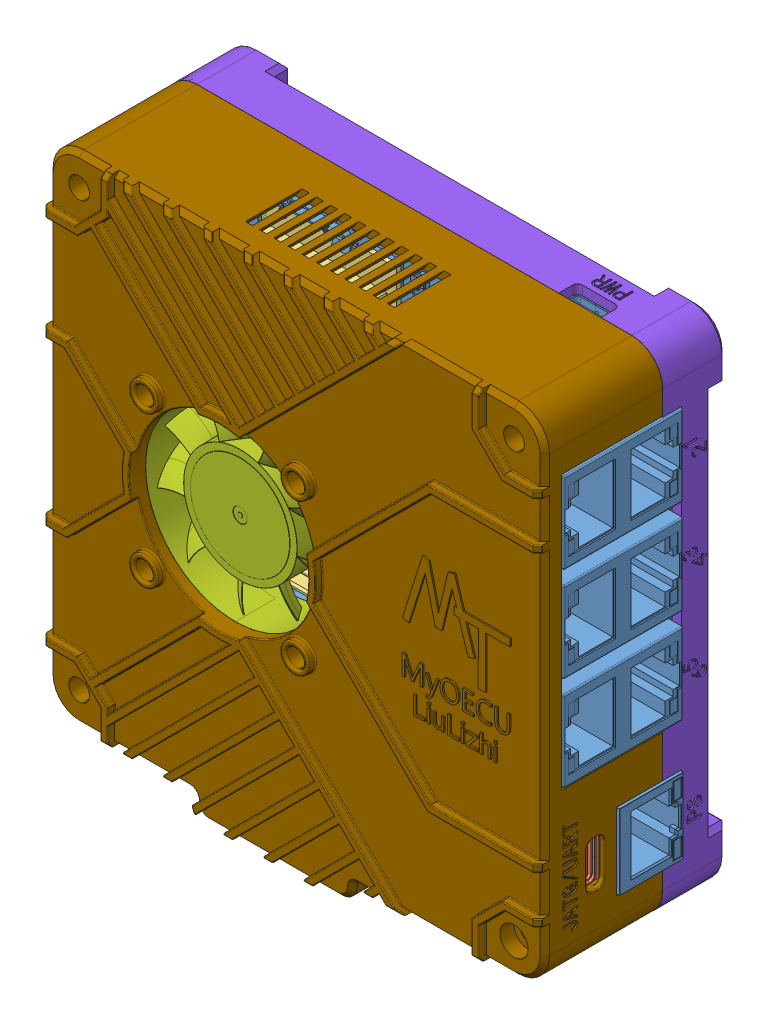
SolidWorks assembly MyOECU_装配1, configuration 默认. Lengths in mm.
Overall size (110.76 109.2 40.07).
11 component instances, 9 part files, 21 mates.
Components (placement in the parent):
- OECU_BASE-1: OECU_BASE [默认] at (25.1566 -137.4235 46.5251) size (110.76 104.44 29.35)
- JTAG-1: JTAG [默认] at (121.0536 -114.4556 17.2477) size (47.13 32.25 13.3)
- ZYNQ_CORE-1: ZYNQ_CORE [1.5V] at (53.9162 -68.6655 52.5951) x (0 -1 0) z (-1 0 0) size (67.6 9 30)
- Column_M3x16-1: Column_M3x16 [Predeterminado] at (93.1566 -123.4235 52.5251) x (1 0 0) z (0 -1 0) size (5.77 15 5)
- Column_M3x16-2: Column_M3x16 [Predeterminado] at (131.1566 -123.4235 52.5251) x (1 0 0) z (0 -1 0) size (5.77 15 5)
- Column_M3x16-3: Column_M3x16 [Predeterminado] at (131.1566 -99.4235 52.5251) x (1 0 0) z (0 -1 0) size (5.77 15 5)
- PinSocket7_2.54-1: PinSocket7_2.54 [默认] at (87.8883 -116.9162 44.9359) x (0 1 0) z (0 0 -1) size (10.13 17.78 5.84)
- OLED-1: OLED [Default] at (93.9183 -129.4462 69.9659) x (-1 0 0) z (0 0 1) size (27.3 11.8 27.8)
- 4010_FAN-1: 4010_FAN [默认] at (70.1566 -77.4235 62.4359) x (0 -1 0) z (-1 0 0) size (43.27 11 40)
- 外壳_底壳-2: 外壳_底壳 [默认] at (0.001 -127.4235 39.9359) x (1 0 0) z (0 -1 0) size (105 14.95 109.2)
- 外壳_上壳-1: 外壳_上壳 [默认] at (-5.4222 -123.4235 73.4359) x (1 0 0) z (0 -1 0) size (105 30.2 109.2)
Mates (geometry in assembly coordinates):
- 同心2: concentric aligned: cylinder of OECU_BASE-1 through (131.1566 -123.4235 44.9359) axis (0 0 -1) radius 1.6; cylinder of JTAG-1 through (131.1566 -123.4235 61.5251) axis (0 0 -1) radius 1.6
- 重合2: coincident: plane of OECU_BASE-1 through (55.9626 -100.8705 52.0951) normal (0 0 1); plane of ZYNQ_CORE-1 through (83.9162 -34.8655 52.0951) normal (0 0 -1)
- 重合3: coincident anti-aligned: plane of OECU_BASE-1 through (49.1126 -60.1655 54.5751) normal (0 -1 0); plane of ZYNQ_CORE-1 through (53.9162 -60.1655 52.0951) normal (0 1 0)
- 重合4: coincident anti-aligned: plane of OECU_BASE-1 through (39.1566 -127.4235 46.5251) normal (0 0 1); plane of Column_M3x16-1 through (93.1566 -123.4235 46.5251) normal (0 0 -1)
- 同心3: concentric aligned: cylinder of JTAG-1 through (93.1566 -123.4235 61.5251) axis (0 0 -1) radius 1.6; cylinder of Column_M3x16-1 through (93.1566 -123.4235 58.5251) axis (0 0 -1) radius 1.5
- 同心4: concentric aligned: cylinder of JTAG-1 through (131.1566 -123.4235 61.5251) axis (0 0 -1) radius 1.6; cylinder of Column_M3x16-2 through (131.1566 -123.4235 58.5251) axis (0 0 -1) radius 1.5
- 同心5: concentric aligned: cylinder of JTAG-1 through (131.1566 -99.4235 61.5251) axis (0 0 -1) radius 1.6; cylinder of Column_M3x16-3 through (131.1566 -99.4235 58.5251) axis (0 0 -1) radius 1.5
- 重合6: coincident anti-aligned: plane of JTAG-1 through (93.1566 -127.5508 61.5251) normal (0 0 -1); plane of Column_M3x16-3 through (131.1566 -99.4235 61.5251) normal (0 0 1)
- 重合7: coincident anti-aligned: plane of JTAG-1 through (93.1566 -127.5508 61.5251) normal (0 0 -1); plane of Column_M3x16-2 through (131.1566 -123.4235 61.5251) normal (0 0 1)
- 重合8: coincident anti-aligned: plane of OECU_BASE-1 through (39.1566 -127.4235 44.9359) normal (0 0 -1); plane of PinSocket7_2.54-1 through (89.1583 -118.4362 44.9359) normal (0 0 1)
- 重合9: coincident anti-aligned: plane of PinSocket7_2.54-1 through (71.3783 -126.9462 42.3959) normal (0 -1 0); plane of OLED-1 through (93.9183 -126.9462 69.9659) normal (0 1 0)
- 重合10: coincident aligned: plane of PinSocket7_2.54-1 through (71.3783 -118.4362 42.3959) normal (0 0 -1); plane of OLED-1 through (73.8183 -126.9462 42.3959) normal (0 0 -1)
- 重合11: coincident aligned: plane of PinSocket7_2.54-1 through (71.3783 -118.4362 44.9359) normal (-1 0 0); plane of OLED-1 through (71.3783 -126.9462 44.8359) normal (-1 0 0)
- 重合12: coincident anti-aligned: plane of OECU_BASE-1 through (39.1566 -127.4235 46.5251) normal (0 0 1); plane of Column_M3x16-2 through (131.1566 -123.4235 46.5251) normal (0 0 -1)
- 距离7: distance = 28.5 mm anti-aligned: plane of 4010_FAN-1 through (70.1566 -77.4235 73.4359) normal (0 0 1); plane of OECU_BASE-1 through (39.1566 -127.4235 44.9359) normal (0 0 -1)
- 距离8: distance = 30 mm aligned: plane of 4010_FAN-1 through (50.1566 -97.4235 62.4359) normal (0 -1 0); plane of OECU_BASE-1 through (131.1566 -127.4235 44.9359) normal (0 -1 0)
- 距离9: distance = 15 mm aligned: plane of OECU_BASE-1 through (35.1566 -123.4235 44.9359) normal (-1 0 0); plane of 4010_FAN-1 through (50.1566 -57.4235 62.4359) normal (-1 0 0)
- 距离10: distance = 3 mm anti-aligned: plane of 外壳_底壳-2 through (0.001 -127.4235 41.9359) normal (0 0 1); plane of OECU_BASE-1 through (39.1566 -127.4235 44.9359) normal (0 0 -1)
- 同心11: concentric aligned: cylinder of OECU_BASE-1 through (39.1566 -123.4235 44.9359) axis (0 0 -1) radius 1.6; cylinder of 外壳_底壳-2 through (39.1566 -123.4235 41.9359) axis (0 0 -1) radius 1.6
- 重合13: coincident anti-aligned: plane of 4010_FAN-1 through (70.1566 -77.4235 73.4359) normal (0 0 1); plane of 外壳_上壳-1 through (39.1566 -123.4235 73.4359) normal (0 0 -1)
- 同心12: concentric aligned: cylinder of 外壳_底壳-2 through (39.1566 -123.4235 41.9359) axis (0 0 -1) radius 1.6; cylinder of 外壳_上壳-1 through (39.1566 -123.4235 75.4359) axis (0 0 -1) radius 1.6
